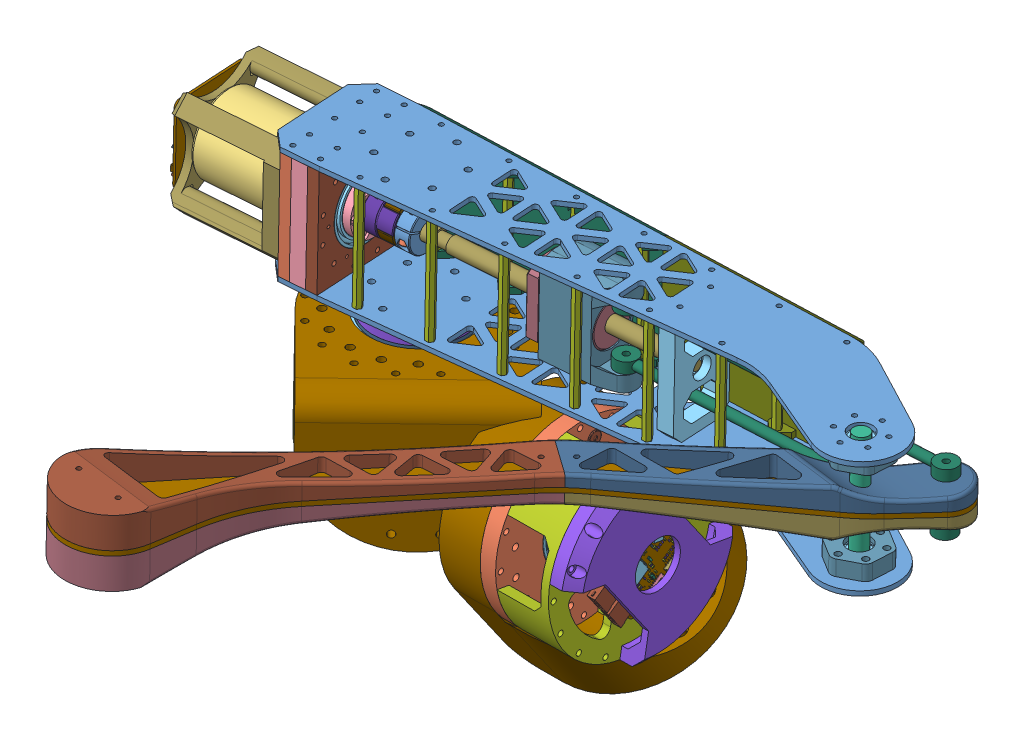
SolidWorks assembly Leg, configuration Default. Lengths in mm. (continued)
Components (placement in the parent): (continued)
- Cycloidal _v3-1: Cycloidal _v3 [Default] at (201.9883 83.8715 287.662) x (0.007254 0.020702 0.999759) z (-0.999974 0 0.007256) size (173.36 87.57 173.15) (continued)
  - M3x20-1: M3x20 [Default] at (43.4726 96.3558 90.1203) x (-0.837193 -0.000334 -0.546908) z (-0.546908 -0.000218 0.837193) size (6 21.2 6)
  - M3x10-1: M3x10 [Default] at (36.5111 25.853 142.5044) x (0.424034 0.000169 -0.905646) z (0.905646 0.000361 0.424034) size (6 11.2 6)
  - m3x60-1: m3x60 [Default] at (17.1068 35.0453 134.2855) x (-0.837193 -0.000334 -0.546908) z (-0.546908 -0.000218 0.837193) size (5.3 63 5.3)
  - m6-1: m6 [Default] at (60.6129 98.6627 108.4832) x (-0.153131 -0.000061 0.988206) z (0.988206 0.000394 0.153131) size (6 16 6)
- Cycloidal _v3-2: Cycloidal _v3 [Default] at (290.9356 44.932 396.0406) x (-0.007136 -0.180415 -0.983565) z (-0.001309 0.983591 -0.18041) size (173.36 87.57 173.15)
  - motor-X83008S.stp-1: motor-X83008S.stp [Default] at (3.9105 88.7742 94.1058) x (0.928336 0.00037 -0.371741) z (0.000399 -1 0) size (114.7 114.7 37.62) (hidden)
    - base.stp-1: base.stp [Default] at (42.0794 12.0269 46.7342) size (91.6 91.6 15.61)
    - stator.stp-1: stator.stp [Default] at (42.0794 12.0269 33.1342) x (0.08493 -0.996387 0) z (0 0 1) size (83 83 8)
    - coil.stp-1: coil.stp [Default] at (39.5332 41.8984 37.1342) x (0.996387 0.08493 0) z (-0.08493 0.996387 0) size (4.4 10.2 10.5)
    - coil.stp-2: coil.stp [Default] at (34.3848 41.0025 37.1342) x (0.966502 0.256661 0) z (-0.256661 0.966502 0) size (4.4 10.2 10.5)
    - coil.stp-3: coil.stp [Default] at (29.4701 39.2261 37.1342) x (0.90725 0.420593 0) z (-0.420593 0.90725 0) size (4.4 10.2 10.5)
    - coil.stp-4: coil.stp [Default] at (24.9386 36.6233 37.1342) x (0.820431 0.571745 0) z (-0.571745 0.820431 0) size (4.4 10.2 10.5)
    - coil.stp-5: coil.stp [Default] at (20.9279 33.2732 37.1342) x (0.708685 0.705525 0) z (-0.705525 0.708685 0) size (4.4 10.2 10.5)
    - coil.stp-6: coil.stp [Default] at (17.5599 29.2775 37.1342) x (0.575405 0.817869 0) z (-0.817869 0.575405 0) size (4.4 10.2 10.5)
    - coil.stp-7: coil.stp [Default] at (14.9368 24.7576 37.1342) x (0.424642 0.905361 0) z (-0.905361 0.424642 0) size (4.4 10.2 10.5)
    - coil.stp-8: coil.stp [Default] at (13.1385 19.8509 37.1342) x (0.260976 0.965345 0) z (-0.965345 0.260976 0) size (4.4 10.2 10.5)
    - coil.stp-9: coil.stp [Default] at (12.2196 14.7066 37.1342) x (0.089381 0.995998 0) z (-0.995998 0.089381 0) size (4.4 10.2 10.5)
    - coil.stp-10: coil.stp [Default] at (12.2079 9.4807 37.1342) x (-0.08493 0.996387 0) z (-0.996387 -0.08493 0) size (4.4 10.2 10.5)
    - coil.stp-11: coil.stp [Default] at (13.1039 4.3323 37.1342) x (-0.256661 0.966502 0) z (-0.966502 -0.256661 0) size (4.4 10.2 10.5)
    - coil.stp-12: coil.stp [Default] at (14.8802 -0.5824 37.1342) x (-0.420593 0.90725 0) z (-0.90725 -0.420593 0) size (4.4 10.2 10.5)
    - coil.stp-13: coil.stp [Default] at (17.483 -5.1139 37.1342) x (-0.571745 0.820431 0) z (-0.820431 -0.571745 0) size (4.4 10.2 10.5)
    - coil.stp-14: coil.stp [Default] at (20.8332 -9.1246 37.1342) x (-0.705525 0.708685 0) z (-0.708685 -0.705525 0) size (4.4 10.2 10.5)
    - coil.stp-15: coil.stp [Default] at (24.8289 -12.4926 37.1342) x (-0.817869 0.575405 0) z (-0.575405 -0.817869 0) size (4.4 10.2 10.5)
    - coil.stp-16: coil.stp [Default] at (29.3487 -15.1157 37.1342) x (-0.905361 0.424642 0) z (-0.424642 -0.905361 0) size (4.4 10.2 10.5)
    - coil.stp-17: coil.stp [Default] at (34.2554 -16.914 37.1342) x (-0.965345 0.260976 0) z (-0.260976 -0.965345 0) size (4.4 10.2 10.5)
    - coil.stp-18: coil.stp [Default] at (39.3998 -17.8329 37.1342) x (-0.995998 0.089381 0) z (-0.089381 -0.995998 0) size (4.4 10.2 10.5)
    - coil.stp-19: coil.stp [Default] at (44.6256 -17.8446 37.1342) x (-0.996387 -0.08493 0) z (0.08493 -0.996387 0) size (4.4 10.2 10.5)
    - coil.stp-20: coil.stp [Default] at (49.7741 -16.9486 37.1342) x (-0.966502 -0.256661 0) z (0.256661 -0.966502 0) size (4.4 10.2 10.5)
    - coil.stp-21: coil.stp [Default] at (54.6887 -15.1723 37.1342) x (-0.90725 -0.420593 0) z (0.420593 -0.90725 0) size (4.4 10.2 10.5)
    - coil.stp-22: coil.stp [Default] at (59.2202 -12.5695 37.1342) x (-0.820431 -0.571745 0) z (0.571745 -0.820431 0) size (4.4 10.2 10.5)
    - coil.stp-23: coil.stp [Default] at (63.2309 -9.2193 37.1342) x (-0.708685 -0.705525 0) z (0.705525 -0.708685 0) size (4.4 10.2 10.5)
    - coil.stp-24: coil.stp [Default] at (66.599 -5.2236 37.1342) x (-0.575405 -0.817869 0) z (0.817869 -0.575405 0) size (4.4 10.2 10.5)
    - coil.stp-25: coil.stp [Default] at (69.222 -0.7038 37.1342) x (-0.424642 -0.905361 0) z (0.905361 -0.424642 0) size (4.4 10.2 10.5)
    - coil.stp-26: coil.stp [Default] at (71.0203 4.2029 37.1342) x (-0.260976 -0.965345 0) z (0.965345 -0.260976 0) size (4.4 10.2 10.5)
    - coil.stp-27: coil.stp [Default] at (71.9392 9.3473 37.1342) x (-0.089381 -0.995998 0) z (0.995998 -0.089381 0) size (4.4 10.2 10.5)
    - coil.stp-28: coil.stp [Default] at (71.9509 14.5731 37.1342) x (0.08493 -0.996387 0) z (0.996387 0.08493 0) size (4.4 10.2 10.5)
    - coil.stp-29: coil.stp [Default] at (71.055 19.7216 37.1342) x (0.256661 -0.966502 0) z (0.966502 0.256661 0) size (4.4 10.2 10.5)
    - coil.stp-30: coil.stp [Default] at (69.2786 24.6362 37.1342) x (0.420593 -0.90725 0) z (0.90725 0.420593 0) size (4.4 10.2 10.5)
    - coil.stp-31: coil.stp [Default] at (66.6758 29.1677 37.1342) x (0.571745 -0.820431 0) z (0.820431 0.571745 0) size (4.4 10.2 10.5)
    - coil.stp-32: coil.stp [Default] at (63.3257 33.1785 37.1342) x (0.705525 -0.708685 0) z (0.708685 0.705525 0) size (4.4 10.2 10.5)
    - coil.stp-33: coil.stp [Default] at (59.33 36.5465 37.1342) x (0.817869 -0.575405 0) z (0.575405 0.817869 0) size (4.4 10.2 10.5)
    - coil.stp-34: coil.stp [Default] at (54.8101 39.1695 37.1342) x (0.905361 -0.424642 0) z (0.424642 0.905361 0) size (4.4 10.2 10.5)
    - coil.stp-35: coil.stp [Default] at (49.9034 40.9678 37.1342) x (0.965345 -0.260976 0) z (0.260976 0.965345 0) size (4.4 10.2 10.5)
    - coil.stp-36: coil.stp [Default] at (44.759 41.8868 37.1342) x (0.995998 -0.089381 0) z (0.089381 0.995998 0) size (4.4 10.2 10.5)
    - rotor.stp-1: rotor.stp [Default] at (42.0794 12.0269 42.1342) x (-0.293442 0.955977 0) z (0 0 -1) size (91.8 91.8 12)
    - outrunner.stp-1: outrunner.stp [Default] at (42.0794 12.0269 30.1342) x (-0.254711 0.967017 0) z (-0.967017 -0.254711 0) size (91.8 17.01 91.8)
    - screw-mount.stp-1: screw-mount.stp [Default] at (38.1314 27.0157 27.1342) x (1 0 0) z (0 0 -1) size (7 7 6.5)
    - screw-mount.stp-2: screw-mount.stp [Default] at (27.0906 8.0789 27.1342) x (1 0 0) z (0 0 -1) size (7 7 6.5)
    - screw-mount.stp-3: screw-mount.stp [Default] at (57.0682 15.9749 27.1342) x (1 0 0) z (0 0 -1) size (7 7 6.5)
    - screw-mount.stp-4: screw-mount.stp [Default] at (46.0274 -2.9618 27.1342) x (1 0 0) z (0 0 -1) size (7 7 6.5)
    - 6702ZZ-bearing-15x21x4.stp-1: 6702ZZ-bearing-15x21x4.stp [Default] at (42.0794 12.0269 43.7342) x (1 0 0) z (0 -1 0) size (21 4 21)
    - 6702ZZ-bearing-15x21x4.stp-2: 6702ZZ-bearing-15x21x4.stp [Default] at (42.0794 12.0269 35.1342) x (1 0 0) z (0 1 0) size (21 4 21)
    - shaft.stp-1: shaft.stp [Default] at (42.0794 12.0269 20.1342) size (16 16 31.6)
    - fix-screw.stp-1: fix-screw.stp [Default] at (42.0794 12.0269 51.7342) x (1 0 0) z (0 0 -1) size (19.67 18.96 12.02)
  - Base_Plate-1: Base_Plate [Default] at (47.4533 68.6574 89.6282) x (-0.992404 -0.000396 0.123023) z (-0.123023 -0.000049 -0.992404) size (39.8 11 39.8)
  - Eccentric_Shaft-1: Eccentric_Shaft [Default] at (60.4961 73.3217 80.3225) x (0.123023 0.000049 0.992404) z (-0.992404 -0.000396 0.123023) size (20 17 17)
    - Eccentric_Shaft_bot-1: Eccentric_Shaft_bot [Default] at (7.6302 12.3409 14.0904) x (1 0 0) z (0 0 -1) size (17 6 17)
    - Eccentric_Shaft_bot-2: Eccentric_Shaft_bot [Default] at (7.6302 12.3409 14.0904) x (-1 0 0) z (0 0 -1) size (17 6 17)
    - Eccentric_Shaft_top-1: Eccentric_Shaft_top [Default] at (7.6302 18.3409 14.0904) x (-1 0 0) z (0 0 -1) size (17 5 17)
  - radial ball bearing_68_iso-39: radial ball bearing_68_iso [ISO 15 RBB - 1860 - 32,SI,NC,32_68] at (47.4409 99.6574 89.6282) x (0.000399 -1 0) z (-0.546908 -0.000218 0.837193) size (10 78 78)
  - radial ball bearing_68_iso-40: radial ball bearing_68_iso [ISO 15 RBB - 1840 - 32,SI,NC,32_68] at (47.4516 72.9574 89.6282) x (-0.000399 1 0) z (0.001003 0 0.999999) size (7 52 52)
  - Base_plate_2-1: Base_plate_2 [Default] at (47.4529 69.6574 89.6282) x (0.712755 0.000284 -0.701413) z (0.701413 0.00028 0.712755) size (115 10 115)
  - m13_bearing-31: m13_bearing [Default] at (-10.4263 95.4017 67.196) x (0.227678 0.000091 0.973736) z (0.973736 0.000388 -0.227678) size (13 16 13)
    - m6-1: m6 [Default] at (8.4921 2.5508 14.8914) size (6 16 6)
    - radial ball bearing_68_iso-1: radial ball bearing_68_iso [ISO 15 RBB - 286 - 10,SI,NC,10_68] at (8.4921 16.0508 14.8914) x (0 1 0) z (0 0 1) size (5 13 13)
    - radial ball bearing_68_iso-2: radial ball bearing_68_iso [ISO 15 RBB - 286 - 10,SI,NC,10_68] at (8.4921 11.0508 14.8914) x (0 1 0) z (0 0 1) size (5 13 13)
  - m13_bearing-32: m13_bearing [Default] at (-13.9908 98.1837 84.3887) x (0.227678 0.000091 0.973736) z (0.973736 0.000388 -0.227678) size (13 16 13)
    - m6-1: m6 [Default] at (8.4921 2.5508 14.8914) size (6 16 6)
    - radial ball bearing_68_iso-1: radial ball bearing_68_iso [ISO 15 RBB - 286 - 10,SI,NC,10_68] at (8.4921 16.0508 14.8914) x (0 1 0) z (0 0 1) size (5 13 13)
    - radial ball bearing_68_iso-2: radial ball bearing_68_iso [ISO 15 RBB - 286 - 10,SI,NC,10_68] at (8.4921 11.0508 14.8914) x (0 1 0) z (0 0 1) size (5 13 13)
  - m13_bearing-34: m13_bearing [Default] at (13.4541 98.1947 126.1847) x (0.227678 0.000091 0.973736) z (0.973736 0.000388 -0.227678) size (13 16 13)
    - m6-1: m6 [Default] at (8.4921 2.5508 14.8914) size (6 16 6)
    - radial ball bearing_68_iso-1: radial ball bearing_68_iso [ISO 15 RBB - 286 - 10,SI,NC,10_68] at (8.4921 16.0508 14.8914) x (0 1 0) z (0 0 1) size (5 13 13)
    - radial ball bearing_68_iso-2: radial ball bearing_68_iso [ISO 15 RBB - 286 - 10,SI,NC,10_68] at (8.4921 11.0508 14.8914) x (0 1 0) z (0 0 1) size (5 13 13)
  - m13_bearing-35: m13_bearing [Default] at (-1.0662 98.1889 116.3132) x (0.227678 0.000091 0.973736) z (0.973736 0.000388 -0.227678) size (13 16 13)
    - m6-1: m6 [Default] at (8.4921 2.5508 14.8914) size (6 16 6)
    - radial ball bearing_68_iso-1: radial ball bearing_68_iso [ISO 15 RBB - 286 - 10,SI,NC,10_68] at (8.4921 16.0508 14.8914) x (0 1 0) z (0 0 1) size (5 13 13)
    - radial ball bearing_68_iso-2: radial ball bearing_68_iso [ISO 15 RBB - 286 - 10,SI,NC,10_68] at (8.4921 11.0508 14.8914) x (0 1 0) z (0 0 1) size (5 13 13)
  - m13_bearing-36: m13_bearing [Default] at (-10.7036 98.185 101.6364) x (0.227678 0.000091 0.973736) z (0.973736 0.000388 -0.227678) size (13 16 13)
    - m6-1: m6 [Default] at (8.4921 2.5508 14.8914) size (6 16 6)
    - radial ball bearing_68_iso-1: radial ball bearing_68_iso [ISO 15 RBB - 286 - 10,SI,NC,10_68] at (8.4921 16.0508 14.8914) x (0 1 0) z (0 0 1) size (5 13 13)
    - radial ball bearing_68_iso-2: radial ball bearing_68_iso [ISO 15 RBB - 286 - 10,SI,NC,10_68] at (8.4921 11.0508 14.8914) x (0 1 0) z (0 0 1) size (5 13 13)
  - m13_bearing-1: m13_bearing [Default] at (-0.4494 98.1891 62.778) x (0.736525 0.000294 0.676411) z (0.676411 0.00027 -0.736525) size (13 16 13)
    - m6-1: m6 [Default] at (8.4921 2.5508 14.8914) size (6 16 6)
    - radial ball bearing_68_iso-1: radial ball bearing_68_iso [ISO 15 RBB - 286 - 10,SI,NC,10_68] at (8.4921 16.0508 14.8914) x (0 1 0) z (0 0 1) size (5 13 13)
    - radial ball bearing_68_iso-2: radial ball bearing_68_iso [ISO 15 RBB - 286 - 10,SI,NC,10_68] at (8.4921 11.0508 14.8914) x (0 1 0) z (0 0 1) size (5 13 13)
  - m13_bearing-2: m13_bearing [Default] at (48.5236 98.2087 124.7001) x (0.120271 0.000048 0.992741) z (0.992741 0.000396 -0.120271) size (13 16 13)
    - m6-1: m6 [Default] at (8.4921 2.5508 14.8914) size (6 16 6)
    - radial ball bearing_68_iso-1: radial ball bearing_68_iso [ISO 15 RBB - 286 - 10,SI,NC,10_68] at (8.4921 16.0508 14.8914) x (0 1 0) z (0 0 1) size (5 13 13)
    - radial ball bearing_68_iso-2: radial ball bearing_68_iso [ISO 15 RBB - 286 - 10,SI,NC,10_68] at (8.4921 11.0508 14.8914) x (0 1 0) z (0 0 1) size (5 13 13)
  - m13_bearing-3: m13_bearing [Default] at (32.5019 98.2023 52.3604) x (0.833889 0.000333 0.551933) z (0.551932 0.00022 -0.833889) size (13 16 13)
    - m6-1: m6 [Default] at (8.4921 2.5508 14.8914) size (6 16 6)
    - radial ball bearing_68_iso-1: radial ball bearing_68_iso [ISO 15 RBB - 286 - 10,SI,NC,10_68] at (8.4921 16.0508 14.8914) x (0 1 0) z (0 0 1) size (5 13 13)
    - radial ball bearing_68_iso-2: radial ball bearing_68_iso [ISO 15 RBB - 286 - 10,SI,NC,10_68] at (8.4921 11.0508 14.8914) x (0 1 0) z (0 0 1) size (5 13 13)
  - m13_bearing-4: m13_bearing [Default] at (77.3632 98.2202 81.8307) x (0.022268 0.000009 0.999752) z (0.999752 0.000399 -0.022268) size (13 16 13)
    - m6-1: m6 [Default] at (8.4921 2.5508 14.8914) size (6 16 6)
    - radial ball bearing_68_iso-1: radial ball bearing_68_iso [ISO 15 RBB - 286 - 10,SI,NC,10_68] at (8.4921 16.0508 14.8914) x (0 1 0) z (0 0 1) size (5 13 13)
    - radial ball bearing_68_iso-2: radial ball bearing_68_iso [ISO 15 RBB - 286 - 10,SI,NC,10_68] at (8.4921 11.0508 14.8914) x (0 1 0) z (0 0 1) size (5 13 13)
  - m13_bearing-5: m13_bearing [Default] at (73.5091 98.2186 99.5852) x (0.059133 0.000024 0.99825) z (0.99825 0.000398 -0.059133) size (13 16 13)
    - m6-1: m6 [Default] at (8.4921 2.5508 14.8914) size (6 16 6)
    - radial ball bearing_68_iso-1: radial ball bearing_68_iso [ISO 15 RBB - 286 - 10,SI,NC,10_68] at (8.4921 16.0508 14.8914) x (0 1 0) z (0 0 1) size (5 13 13)
    - radial ball bearing_68_iso-2: radial ball bearing_68_iso [ISO 15 RBB - 286 - 10,SI,NC,10_68] at (8.4921 11.0508 14.8914) x (0 1 0) z (0 0 1) size (5 13 13)
  - m13_bearing-6: m13_bearing [Default] at (13.4333 98.1947 47.0643) x (0.451561 0.00018 0.89224) z (0.89224 0.000356 -0.451561) size (13 16 13)
    - m6-1: m6 [Default] at (8.4921 2.5508 14.8914) size (6 16 6)
    - radial ball bearing_68_iso-1: radial ball bearing_68_iso [ISO 15 RBB - 286 - 10,SI,NC,10_68] at (8.4921 16.0508 14.8914) x (0 1 0) z (0 0 1) size (5 13 13)
    - radial ball bearing_68_iso-2: radial ball bearing_68_iso [ISO 15 RBB - 286 - 10,SI,NC,10_68] at (8.4921 11.0508 14.8914) x (0 1 0) z (0 0 1) size (5 13 13)
  - m13_bearing-7: m13_bearing [Default] at (57.1526 98.2121 32.9496) x (-0.545813 -0.000218 0.837907) z (0.837907 0.000334 0.545813) size (13 16 13)
    - m6-1: m6 [Default] at (8.4921 2.5508 14.8914) size (6 16 6)
    - radial ball bearing_68_iso-1: radial ball bearing_68_iso [ISO 15 RBB - 286 - 10,SI,NC,10_68] at (8.4921 16.0508 14.8914) x (0 1 0) z (0 0 1) size (5 13 13)
    - radial ball bearing_68_iso-2: radial ball bearing_68_iso [ISO 15 RBB - 286 - 10,SI,NC,10_68] at (8.4921 11.0508 14.8914) x (0 1 0) z (0 0 1) size (5 13 13)
  - m13_bearing-8: m13_bearing [Default] at (73.1034 98.2185 66.7178) x (0.158553 0.000063 0.98735) z (0.98735 0.000394 -0.158553) size (13 16 13)
    - m6-1: m6 [Default] at (8.4921 2.5508 14.8914) size (6 16 6)
    - radial ball bearing_68_iso-1: radial ball bearing_68_iso [ISO 15 RBB - 286 - 10,SI,NC,10_68] at (8.4921 16.0508 14.8914) x (0 1 0) z (0 0 1) size (5 13 13)
    - radial ball bearing_68_iso-2: radial ball bearing_68_iso [ISO 15 RBB - 286 - 10,SI,NC,10_68] at (8.4921 11.0508 14.8914) x (0 1 0) z (0 0 1) size (5 13 13)
  - m13_bearing-9: m13_bearing [Default] at (74.5316 98.219 41.6624) x (-0.687134 -0.000274 0.72653) z (0.72653 0.00029 0.687134) size (13 16 13)
    - m6-1: m6 [Default] at (8.4921 2.5508 14.8914) size (6 16 6)
    - radial ball bearing_68_iso-1: radial ball bearing_68_iso [ISO 15 RBB - 286 - 10,SI,NC,10_68] at (8.4921 16.0508 14.8914) x (0 1 0) z (0 0 1) size (5 13 13)
    - radial ball bearing_68_iso-2: radial ball bearing_68_iso [ISO 15 RBB - 286 - 10,SI,NC,10_68] at (8.4921 11.0508 14.8914) x (0 1 0) z (0 0 1) size (5 13 13)
  - m13_bearing-11: m13_bearing [Default] at (30.0113 98.2013 136.2104) x (0.57351 0.000229 0.819198) z (0.819198 0.000327 -0.57351) size (13 16 13)
    - m6-1: m6 [Default] at (8.4921 2.5508 14.8914) size (6 16 6)
    - radial ball bearing_68_iso-1: radial ball bearing_68_iso [ISO 15 RBB - 286 - 10,SI,NC,10_68] at (8.4921 16.0508 14.8914) x (0 1 0) z (0 0 1) size (5 13 13)
    - radial ball bearing_68_iso-2: radial ball bearing_68_iso [ISO 15 RBB - 286 - 10,SI,NC,10_68] at (8.4921 11.0508 14.8914) x (0 1 0) z (0 0 1) size (5 13 13)
  - m13_bearing-12: m13_bearing [Default] at (62.5932 98.2143 116.7506) x (0.22335 0.000089 0.974738) z (0.974738 0.000389 -0.22335) size (13 16 13)
    - m6-1: m6 [Default] at (8.4921 2.5508 14.8914) size (6 16 6)
    - radial ball bearing_68_iso-1: radial ball bearing_68_iso [ISO 15 RBB - 286 - 10,SI,NC,10_68] at (8.4921 16.0508 14.8914) x (0 1 0) z (0 0 1) size (5 13 13)
    - radial ball bearing_68_iso-2: radial ball bearing_68_iso [ISO 15 RBB - 286 - 10,SI,NC,10_68] at (8.4921 11.0508 14.8914) x (0 1 0) z (0 0 1) size (5 13 13)
  - M3x4x4.2_brass_insert-22: M3x4x4.2_brass_insert [Default] at (43.4837 68.6558 90.1203) x (0.984609 0.000393 -0.174769) z (0.174769 0.00007 0.984609) size (4 4 4)
  - M3x4x4.2_brass_insert-23: M3x4x4.2_brass_insert [Default] at (51.4229 68.659 89.1361) x (0.984609 0.000393 -0.174769) z (0.174769 0.00007 0.984609) size (4 4 4)
  - radial ball bearing_68_iso-44: radial ball bearing_68_iso [ISO 15 RBB - 1715 - 26,SI,NC,26_68] at (47.2636 81.6573 88.1396) x (0.000399 -1 0) z (0.171535 0.000068 0.985178) size (4 21 21)
  - radial ball bearing_68_iso-45: radial ball bearing_68_iso [ISO 15 RBB - 1715 - 26,SI,NC,26_68] at (47.4429 94.6574 89.6282) x (0.000399 -1 0) z (0.819169 0.000327 0.573552) size (4 21 21)
  - radial ball bearing_68_iso-46: radial ball bearing_68_iso [ISO 15 RBB - 1715 - 26,SI,NC,26_68] at (47.6295 89.6575 91.1168) x (-0.000399 1 0) z (0 0 1) size (4 21 21)
  - foc-motor-controller.step-1: foc-motor-controller.step [Default] at (47.4677 32.6574 89.6282) x (0.701413 0.00028 0.712755) z (0.000399 -1 0) size (57.23 50 8.13)
    - RTA0040B.step-1: RTA0040B.step [Default] at (12.5014 -1.6986 1.595) x (-0.707107 -0.707107 0) z (0 0 1) size (6 6 1)
      - FRAME.step-1: FRAME.step [Default] x (1 0 0) z (0 -1 0) size (6 0.2 6)
        - SOLID.step-1: SOLID.step [Default] at origin size (0.4 0.2 0.22)
        - SOLID-0.step-1: SOLID-0.step [Default] at origin size (0.4 0.2 0.22)
        - SOLID-1.step-1: SOLID-1.step [Default] at origin size (0.4 0.2 0.22)
        - SOLID-2.step-1: SOLID-2.step [Default] at origin size (0.4 0.2 0.22)
        - SOLID-3.step-1: SOLID-3.step [Default] at origin size (0.4 0.2 0.22)
        - SOLID-4.step-1: SOLID-4.step [Default] at origin size (0.4 0.2 0.22)
        - SOLID-5.step-1: SOLID-5.step [Default] at origin size (0.4 0.2 0.22)
        - SOLID-6.step-1: SOLID-6.step [Default] at origin size (0.4 0.2 0.22)
        - SOLID-7.step-1: SOLID-7.step [Default] at origin size (0.4 0.2 0.22)
        - SOLID-8.step-1: SOLID-8.step [Default] at origin size (0.4 0.2 0.22)
        - SOLID-9.step-1: SOLID-9.step [Default] at origin size (0.22 0.2 0.4)
        - SOLID-10.step-1: SOLID-10.step [Default] at origin size (0.22 0.2 0.4)
        - SOLID-11.step-1: SOLID-11.step [Default] at origin size (0.22 0.2 0.4)
        - SOLID-12.step-1: SOLID-12.step [Default] at origin size (0.22 0.2 0.4)
        - SOLID-13.step-1: SOLID-13.step [Default] at origin size (0.22 0.2 0.4)
        - SOLID-14.step-1: SOLID-14.step [Default] at origin size (0.22 0.2 0.4)
        - SOLID-15.step-1: SOLID-15.step [Default] at origin size (0.22 0.2 0.4)
        - SOLID-16.step-1: SOLID-16.step [Default] at origin size (0.22 0.2 0.4)
        - SOLID-17.step-1: SOLID-17.step [Default] at origin size (4.15 0.2 4.15)
        - SOLID-18.step-1: SOLID-18.step [Default] at origin size (0.28 0.1 0.28)
        - SOLID-19.step-1: SOLID-19.step [Default] at origin size (0.28 0.1 0.28)
        - SOLID-20.step-1: SOLID-20.step [Default] at origin size (0.28 0.1 0.28)
        - SOLID-21.step-1: SOLID-21.step [Default] at origin size (0.28 0.1 0.28)
        - SOLID-22.step-1: SOLID-22.step [Default] at origin size (0.4 0.2 0.22)
        - SOLID-23.step-1: SOLID-23.step [Default] at origin size (0.4 0.2 0.22)
        - SOLID-24.step-1: SOLID-24.step [Default] at origin size (0.4 0.2 0.22)
        - SOLID-25.step-1: SOLID-25.step [Default] at origin size (0.4 0.2 0.22)
        - SOLID-26.step-1: SOLID-26.step [Default] at origin size (0.4 0.2 0.22)
        - SOLID-27.step-1: SOLID-27.step [Default] at origin size (0.4 0.2 0.22)
        - SOLID-28.step-1: SOLID-28.step [Default] at origin size (0.4 0.2 0.22)
        - SOLID-29.step-1: SOLID-29.step [Default] at origin size (0.4 0.2 0.22)
        - SOLID-30.step-1: SOLID-30.step [Default] at origin size (0.4 0.2 0.22)
        - SOLID-31.step-1: SOLID-31.step [Default] at origin size (0.4 0.2 0.22)
        - SOLID-32.step-1: SOLID-32.step [Default] at origin size (0.22 0.2 0.4)
        - SOLID-33.step-1: SOLID-33.step [Default] at origin size (0.22 0.2 0.4)
        - SOLID-34.step-1: SOLID-34.step [Default] at origin size (0.22 0.2 0.4)
        - SOLID-35.step-1: SOLID-35.step [Default] at origin size (0.22 0.2 0.4)
        - SOLID-36.step-1: SOLID-36.step [Default] at origin size (0.22 0.2 0.4)
        - SOLID-37.step-1: SOLID-37.step [Default] at origin size (0.22 0.2 0.4)
        - SOLID-38.step-1: SOLID-38.step [Default] at origin size (0.22 0.2 0.4)
        - SOLID-39.step-1: SOLID-39.step [Default] at origin size (0.22 0.2 0.4)
        - SOLID-40.step-1: SOLID-40.step [Default] at origin size (0.22 0.2 0.4)
        - SOLID-41.step-1: SOLID-41.step [Default] at origin size (0.22 0.2 0.4)
        - SOLID-42.step-1: SOLID-42.step [Default] at origin size (0.22 0.2 0.4)
        - SOLID-43.step-1: SOLID-43.step [Default] at origin size (0.22 0.2 0.4)
      - BODY.step-1: BODY.step [Default] at (0 0 0.025) x (1 0 0) z (0 -1 0) size (6 0.97 6)
    - Resonator_SMD_Murata_CSTxExxV-3Pin_3.0x1.1mm.step-1: Resonator_SMD_Murata_CSTxExxV-3Pin_3.0x1.1mm.step [Default] at (1.8 -7 1.595) x (0 1 0) z (0 0 1) size (3.2 1.35 0.9)
    - C_0603_1608Metric.step-1: C_0603_1608Metric.step [Default] at (6.2 -16.8 1.595) x (0 -1 0) z (0 0 1) size (1.6 0.8 0.8)
    - R_0603_1608Metric.step-1: R_0603_1608Metric.step [Default] at (11.8 -7.375 1.595) x (0 1 0) z (0 0 1) size (1.6 0.8 0.45)
    - R_0603_1608Metric.step-2: R_0603_1608Metric.step [Default] at (13.8 -16.8 1.595) x (0 1 0) z (0 0 1) size (1.6 0.8 0.45)
    - R_0603_1608Metric.step-3: R_0603_1608Metric.step [Default] at (18.1 -5.36 1.595) size (1.6 0.8 0.45)
    - C_0603_1608Metric.step-2: C_0603_1608Metric.step [Default] at (2.6 -0.5 1.595) x (0 -1 0) z (0 0 1) size (1.6 0.8 0.8)
    - R_0603_1608Metric.step-4: R_0603_1608Metric.step [Default] at (14.6 -11.3 1.595) x (0 1 0) z (0 0 1) size (1.6 0.8 0.45)
    - L_APV_ANR4020.step-1: L_APV_ANR4020.step [Default] at (22.3 -13.7 1.595) x (0 -1 0) z (0 0 1) size (4.02 4 2)
    - C_0603_1608Metric.step-3: C_0603_1608Metric.step [Default] at (0.3 -12.6 1.595) x (-1 0 0) z (0 0 1) size (1.6 0.8 0.8)
    - C_1206_3216Metric.step-1: C_1206_3216Metric.step [Default] at (15.7 11 1.595) x (0 1 0) z (0 0 1) size (3.2 1.6 1.6)
    - C_0603_1608Metric.step-4: C_0603_1608Metric.step [Default] at (0.3 -9.6 1.595) size (1.6 0.8 0.8)
    - R_0603_1608Metric.step-5: R_0603_1608Metric.step [Default] at (12.3 -16.8 1.595) x (0 1 0) z (0 0 1) size (1.6 0.8 0.45)
    - C_0603_1608Metric.step-5: C_0603_1608Metric.step [Default] at (-0.3 -16.6 1.595) x (0 1 0) z (0 0 1) size (1.6 0.8 0.8)
    - R_0603_1608Metric.step-6: R_0603_1608Metric.step [Default] at (10.9 4.1 1.595) size (1.6 0.8 0.45)
    - C_1206_3216Metric.step-2: C_1206_3216Metric.step [Default] at (6.3 11 1.595) x (0 1 0) z (0 0 1) size (3.2 1.6 1.6)
    - XT30PW_2_2_-M.G.B.step-1: XT30PW_2_2_-M.G.B.step [Default] at (-20.5 9.5 1.595) x (0 -1 0) z (-1 0 0) size (15.5 7.1 12.53)
    - R_0603_1608Metric.step-7: R_0603_1608Metric.step [Default] at (0.3 -11.1 1.595) size (1.6 0.8 0.45)
    - C_0603_1608Metric.step-6: C_0603_1608Metric.step [Default] at (19 -0.4 1.595) x (-0.707107 -0.707107 0) z (0 0 1) size (1.6 0.8 0.8)
    - C_1206_3216Metric.step-3: C_1206_3216Metric.step [Default] at (13.3 11 1.595) x (0 1 0) z (0 0 1) size (3.2 1.6 1.6)
    - R_0603_1608Metric.step-8: R_0603_1608Metric.step [Default] at (10.2 -7.375 1.595) x (0 -1 0) z (0 0 1) size (1.6 0.8 0.45)
    - JST_GH_SM08B-GHS-TB_1x08-1MP_P1.25mm_Horizontal.step-1: JST_GH_SM08B-GHS-TB_1x08-1MP_P1.25mm_Horizontal.step [Default] at (10 -22 1.595) size (13.25 4.95 4.25)
    - C_1206_3216Metric.step-4: C_1206_3216Metric.step [Default] at (-12.3 11 1.595) x (0 1 0) z (0 0 1) size (3.2 1.6 1.6)
    - JST_GH_SM06B-GHS-TB_1x06-1MP_P1.25mm_Horizontal.step-1: JST_GH_SM06B-GHS-TB_1x06-1MP_P1.25mm_Horizontal.step [Default] at (-4.3 -22 1.595) size (10.75 4.95 4.25)
    - C_0603_1608Metric.step-7: C_0603_1608Metric.step [Default] at (7.3 -4.5 1.595) x (-1 0 0) z (0 0 1) size (1.6 0.8 0.8)
    - R_0603_1608Metric.step-9: R_0603_1608Metric.step [Default] at (18.1 -3.86 1.595) x (-1 0 0) z (0 0 1) size (1.6 0.8 0.45)
    - C_1206_3216Metric.step-5: C_1206_3216Metric.step [Default] at (22.6794 -1.2206 1.595) x (0.707107 -0.707107 0) z (0 0 1) size (3.2 1.6 1.6)
    - R_Array_Convex_4x0402.step-1: R_Array_Convex_4x0402.step [Default] at (6.8 -2.5 1.595) size (1 2 0.35)
    - R_0603_1608Metric.step-10: R_0603_1608Metric.step [Default] at (7.7 -16.8 1.595) x (0 -1 0) z (0 0 1) size (1.6 0.8 0.45)
    - C_1206_3216Metric.step-6: C_1206_3216Metric.step [Default] at (8.7 11 1.595) x (0 1 0) z (0 0 1) size (3.2 1.6 1.6)
    - C_0603_1608Metric.step-8: C_0603_1608Metric.step [Default] at (16.1 -11.3 1.595) x (0 1 0) z (0 0 1) size (1.6 0.8 0.8)
    - SOT-23-5.step-1: SOT-23-5.step [Default] at (-3.1 -16.6 1.595) x (-1 0 0) z (0 0 1) size (2.8 2.9 1.55)
    - C_0603_1608Metric.step-9: C_0603_1608Metric.step [Default] at (17.8 -13.6 1.595) size (1.6 0.8 0.8)
    - R_0603_1608Metric.step-11: R_0603_1608Metric.step [Default] at (-11.5 -20.3875 1.595) x (0 -1 0) z (0 0 1) size (1.6 0.8 0.45)
    - C_0603_1608Metric.step-10: C_0603_1608Metric.step [Default] at (-12.4 2.3 1.595) x (0 1 0) z (0 0 1) size (1.6 0.8 0.8)
    - C_1206_3216Metric.step-7: C_1206_3216Metric.step [Default] at (18 11 1.595) x (0 1 0) z (0 0 1) size (3.2 1.6 1.6)
    - R_0603_1608Metric.step-12: R_0603_1608Metric.step [Default] at (-10.8105 -14.9971 1.595) x (-1 0 0) z (0 0 1) size (1.6 0.8 0.45)
    - C_0603_1608Metric.step-11: C_0603_1608Metric.step [Default] at (-13.8 -9.4 1.595) x (-1 0 0) z (0 0 1) size (1.6 0.8 0.8)
    - R_0603_1608Metric.step-13: R_0603_1608Metric.step [Default] at (-23.15 -14.5 1.595) x (-1 0 0) z (0 0 1) size (1.6 0.8 0.45)
    - C_0603_1608Metric.step-12: C_0603_1608Metric.step [Default] at (1.1 -0.2 1.595) x (0 1 0) z (0 0 1) size (1.6 0.8 0.8)
    - D_0805_2012Metric.step-1: D_0805_2012Metric.step [Default] at (22.9 -9.6 1.595) x (0 1 0) z (0 0 1) size (2 1.27 0.8)
    - C_0603_1608Metric.step-13: C_0603_1608Metric.step [Default] at (-7.8 3.775 1.595) x (0 -1 0) z (0 0 1) size (1.6 0.8 0.8)
    - R_0603_1608Metric.step-14: R_0603_1608Metric.step [Default] at (-6.4 -12.825 1.595) x (0 1 0) z (0 0 1) size (1.6 0.8 0.45)
    - L_0603_1608Metric.step-1: L_0603_1608Metric.step [Default] at (-10.1 3 1.595) size (1.6 0.8 0.8)
    - C_0603_1608Metric.step-14: C_0603_1608Metric.step [Default] at (17.9 0.7 1.595) x (-0.707107 -0.707107 0) z (0 0 1) size (1.6 0.8 0.8)
    - HVSSOP-10.step-1: HVSSOP-10.step [Default] at (18.6 -9.6 1.595) x (0 -1 0) z (-1 0 0) size (4.9 1.1 3)
    - C_0603_1608Metric.step-15: C_0603_1608Metric.step [Default] at (7.9 4.1 1.595) x (-1 0 0) z (0 0 1) size (1.6 0.8 0.8)
    - C_0603_1608Metric.step-16: C_0603_1608Metric.step [Default] at (21.1 -9.6 1.595) x (0 -1 0) z (0 0 1) size (1.6 0.8 0.8)
    - R_0603_1608Metric.step-15: R_0603_1608Metric.step [Default] at (-10.8105 -11.9971 1.595) x (-1 0 0) z (0 0 1) size (1.6 0.8 0.45)
    - R_0603_1608Metric.step-16: R_0603_1608Metric.step [Default] at (-18.2 -17.4 1.595) size (1.6 0.8 0.45)
    - C_1206_3216Metric.step-8: C_1206_3216Metric.step [Default] at (-3 11 1.595) x (0 1 0) z (0 0 1) size (3.2 1.6 1.6)
    - R_0603_1608Metric.step-17: R_0603_1608Metric.step [Default] at (-16.9 -20.4 1.595) x (0 -1 0) z (0 0 1) size (1.6 0.8 0.45)
    - R_0603_1608Metric.step-18: R_0603_1608Metric.step [Default] at (-13.3 -20.3875 1.595) x (0 -1 0) z (0 0 1) size (1.6 0.8 0.45)
    - R_0603_1608Metric.step-19: R_0603_1608Metric.step [Default] at (-15.1 -20.3875 1.595) x (0 -1 0) z (0 0 1) size (1.6 0.8 0.45)
    - C_0603_1608Metric.step-17: C_0603_1608Metric.step [Default] at (15.5 -14.4 1.595) x (0 -1 0) z (0 0 1) size (1.6 0.8 0.8)
    - LED_0603_1608Metric.step-1: LED_0603_1608Metric.step [Default] at (-11.5 -23.3875 1.595) x (0 1 0) z (0 0 1) size (1.6 0.8 1.1)
    - C_0805_2012Metric.step-1: C_0805_2012Metric.step [Default] at (19.95 -17 1.595) size (2 1.25 1.25)
    - D_SMB.step-1: D_SMB.step [Default] at (-16.5 11.208 1.595) x (0 -1 0) z (0 0 1) size (5.3 3.55 2.15)
    - C_1206_3216Metric.step-9: C_1206_3216Metric.step [Default] at (-5.3 11 1.595) x (0 1 0) z (0 0 1) size (3.2 1.6 1.6)
    - XT30PW_2_2_-M.G.B.step-2: XT30PW_2_2_-M.G.B.step [Default] at (-20.5 -6.5 1.595) x (0 -1 0) z (-1 0 0) size (15.5 7.1 12.53)
    - C_1206_3216Metric.step-10: C_1206_3216Metric.step [Default] at (1.7 11 1.595) x (0 1 0) z (0 0 1) size (3.2 1.6 1.6)
    - C_1206_3216Metric.step-11: C_1206_3216Metric.step [Default] at (11 11 1.595) x (0 1 0) z (0 0 1) size (3.2 1.6 1.6)
    - C_0603_1608Metric.step-18: C_0603_1608Metric.step [Default] at (-6.3 3.775 1.595) x (0 -1 0) z (0 0 1) size (1.6 0.8 0.8)
    - C_0603_1608Metric.step-19: C_0603_1608Metric.step [Default] at (16.8686 1.7314 1.595) x (0.707107 0.707107 0) z (0 0 1) size (1.6 0.8 0.8)
    - C_0603_1608Metric.step-20: C_0603_1608Metric.step [Default] at (-15.0105 -11.1 1.595) size (1.6 0.8 0.8)
    - C_1206_3216Metric.step-12: C_1206_3216Metric.step [Default] at (-7.7 11 1.595) x (0 1 0) z (0 0 1) size (3.2 1.6 1.6)
    - C_0603_1608Metric.step-21: C_0603_1608Metric.step [Default] at (-18.2 -15.8 1.595) size (1.6 0.8 0.8)
    - C_0603_1608Metric.step-22: C_0603_1608Metric.step [Default] at (-2.1 -11.3 1.595) x (0 -1 0) z (0 0 1) size (1.6 0.8 0.8)
    - C_0603_1608Metric.step-23: C_0603_1608Metric.step [Default] at (-10.8105 -13.4971 1.595) size (1.6 0.8 0.8)
    - C_1206_3216Metric.step-13: C_1206_3216Metric.step [Default] at (4 11 1.595) x (0 1 0) z (0 0 1) size (3.2 1.6 1.6)
    - R_0603_1608Metric.step-20: R_0603_1608Metric.step [Default] at (16 -17.8 1.595) x (0 1 0) z (0 0 1) size (1.6 0.8 0.45)
    - Texas_S-PVSON-N8.step-1: Texas_S-PVSON-N8.step [Default] at (-14.4105 -13.7 1.595) x (-1 0 0) z (0 0 1) size (3 2.98 0.92)
    - C_1206_3216Metric.step-14: C_1206_3216Metric.step [Default] at (21 -2.9 1.595) x (0.707107 -0.707107 0) z (0 0 1) size (3.2 1.6 1.6)
    - C_0603_1608Metric.step-24: C_0603_1608Metric.step [Default] at (-5.9 -16.6 1.595) x (0 1 0) z (0 0 1) size (1.6 0.8 0.8)
    - C_0603_1608Metric.step-25: C_0603_1608Metric.step [Default] at (-3.1 -14.1 1.595) size (1.6 0.8 0.8)
    - R_0603_1608Metric.step-21: R_0603_1608Metric.step [Default] at (7.2 -7.375 1.595) x (0 -1 0) z (0 0 1) size (1.6 0.8 0.45)
    - C_1206_3216Metric.step-15: C_1206_3216Metric.step [Default] at (-0.7 11 1.595) x (0 1 0) z (0 0 1) size (3.2 1.6 1.6)
    - LQFP-64_10x10mm_P0.5mm.step-1: LQFP-64_10x10mm_P0.5mm.step [Default] at (-7 -4.5 1.595) x (-1 0 0) z (0 0 1) size (12 12 1.5)
    - C_0805_2012Metric.step-2: C_0805_2012Metric.step [Default] at (23.35 -17 1.595) x (-1 0 0) z (0 0 1) size (2 1.25 1.25)
    - C_0603_1608Metric.step-26: C_0603_1608Metric.step [Default] at (10.8 -16.8 1.595) x (0 -1 0) z (0 0 1) size (1.6 0.8 0.8)
    - R_0603_1608Metric.step-22: R_0603_1608Metric.step [Default] at (17.5 -17.8 1.595) x (0 -1 0) z (0 0 1) size (1.6 0.8 0.45)
    - C_1206_3216Metric.step-16: C_1206_3216Metric.step [Default] at (20.3 11 1.595) x (0 1 0) z (0 0 1) size (3.2 1.6 1.6)
    - R_0603_1608Metric.step-23: R_0603_1608Metric.step [Default] at (9.2 -16.8 1.595) x (0 -1 0) z (0 0 1) size (1.6 0.8 0.45)
    - C_1206_3216Metric.step-17: C_1206_3216Metric.step [Default] at (-10 11 1.595) x (0 1 0) z (0 0 1) size (3.2 1.6 1.6)
    - R_0603_1608Metric.step-24: R_0603_1608Metric.step [Default] at (17.8 -15.2 1.595) size (1.6 0.8 0.45)
    - C_1206_3216Metric.step-18: C_1206_3216Metric.step [Default] at (19.9 2.6 1.595) x (-0.707107 0.707107 0) z (0 0 1) size (3.2 1.6 1.6)
    - C_0603_1608Metric.step-27: C_0603_1608Metric.step [Default] at (13.4 -7.375 1.595) x (0 -1 0) z (0 0 1) size (1.6 0.8 0.8)
    - R_0603_1608Metric.step-25: R_0603_1608Metric.step [Default] at (8.7 -7.375 1.595) x (0 -1 0) z (0 0 1) size (1.6 0.8 0.45)
    - PQFN-8-EP_6x5mm_P1.27mm_Generic.step-1: PQFN-8-EP_6x5mm_P1.27mm_Generic.step [Default] at (4.9 14.4 -0.085) x (0 1 0) z (0 0 -1) size (6.15 5.15 1.09)
    - C_0805_2012Metric.step-3: C_0805_2012Metric.step [Default] at (-3 8.9 -0.085) x (0 1 0) z (0 0 -1) size (2 1.25 1.25)
    - C_0603_1608Metric.step-28: C_0603_1608Metric.step [Default] at (1.5 -4.3 -0.085) x (0 1 0) z (0 0 -1) size (1.6 0.8 0.8)
    - R_2512_6332Metric.step-1: R_2512_6332Metric.step [Default] at (2.1 8.6 -0.085) x (-1 0 0) z (0 0 -1) size (6.3 3.2 0.6)
    - C_0805_2012Metric.step-4: C_0805_2012Metric.step [Default] at (18.8 8.9 -0.085) x (0 1 0) z (0 0 -1) size (2 1.25 1.25)
    - C_0805_2012Metric.step-5: C_0805_2012Metric.step [Default] at (-5.2 8.901 -0.085) x (0 1 0) z (0 0 -1) size (2 1.25 1.25)
    - PQFN-8-EP_6x5mm_P1.27mm_Generic.step-2: PQFN-8-EP_6x5mm_P1.27mm_Generic.step [Default] at (16.9 14.6 -0.085) x (0 -1 0) z (0 0 -1) size (6.15 5.15 1.09)
    - PQFN-8-EP_6x5mm_P1.27mm_Generic.step-3: PQFN-8-EP_6x5mm_P1.27mm_Generic.step [Default] at (-1.1 14.6 -0.085) x (0 -1 0) z (0 0 -1) size (6.15 5.15 1.09)
    - R_0603_1608Metric.step-26: R_0603_1608Metric.step [Default] at (8.2 8.8 -0.085) x (0 1 0) z (0 0 -1) size (1.6 0.8 0.45)
    - R_2512_6332Metric.step-2: R_2512_6332Metric.step [Default] at (-10.3 8.601 -0.085) x (1 0 0) z (0 0 -1) size (6.3 3.2 0.6)
    - TSSOP-16_4.4x5mm_P0.65mm.step-1: TSSOP-16_4.4x5mm_P0.65mm.step [Default] at (0 0 -0.085) x (-1 0 0) z (0 0 -1) size (6.4 5 1.1)
    - C_0603_1608Metric.step-29: C_0603_1608Metric.step [Default] at (0 -4.25 -0.085) x (0 1 0) z (0 0 -1) size (1.6 0.8 0.8)
    - PQFN-8-EP_6x5mm_P1.27mm_Generic.step-4: PQFN-8-EP_6x5mm_P1.27mm_Generic.step [Default] at (10.9 14.4 -0.085) x (0 1 0) z (0 0 -1) size (6.15 5.15 1.09)
    - R_2512_6332Metric.step-3: R_2512_6332Metric.step [Default] at (13.7 8.6 -0.085) x (1 0 0) z (0 0 -1) size (6.3 3.2 0.6)
    - PQFN-8-EP_6x5mm_P1.27mm_Generic.step-5: PQFN-8-EP_6x5mm_P1.27mm_Generic.step [Default] at (-13.1 14.401 -0.085) x (0 1 0) z (0 0 -1) size (6.15 5.15 1.09)
    - C_0603_1608Metric.step-30: C_0603_1608Metric.step [Default] at (-1.5 -4.3 -0.085) x (0 -1 0) z (0 0 -1) size (1.6 0.8 0.8)
    - PQFN-8-EP_6x5mm_P1.27mm_Generic.step-6: PQFN-8-EP_6x5mm_P1.27mm_Generic.step [Default] at (-7.1 14.601 -0.085) x (0 -1 0) z (0 0 -1) size (6.15 5.15 1.09)
    - foc-motor-controller_PCB.step-1: foc-motor-controller_PCB.step [Default] at origin size (50 50 1.51)
  - hex nut style 1 gradeab_iso-1: hex nut style 1 gradeab_iso [ISO - 4032 - M3 - W - N] at (47.7115 32.6575 59.2236) x (1 0.000399 0) z (0.000399 -1 0) size (5.5 6.35 2.4)
  - Cycloidal_Discs_8308-1: Cycloidal_Discs_8308 [Default] at (-11.9184 124.164 51.5043) x (0.028527 0.000011 0.999593) z (0.999593 0.000399 -0.028527) size (79.25 5 79.73)
    - Cycloidal_Discs-1: Cycloidal_Discs [Default] at (38.3081 39.5303 58.0959) size (79.25 5 79.73)
  - Cycloidal_Discs_8308-2: Cycloidal_Discs_8308 [Default] at (62.1667 47.133 159.1742) x (-0.931329 -0.000371 -0.364178) z (0.364178 0.000145 -0.931329) size (79.25 5 79.73)
    - Cycloidal_Discs-1: Cycloidal_Discs [Default] at (38.3081 39.5303 58.0959) size (79.25 5 79.73)
  - Motor_Cover_v2-2: Motor_Cover_v2 [Default] at (47.4667 35.0574 89.6282) x (0.999968 0.000399 0.00802) z (-0.00802 -0.000003 0.999968) size (115 34.6 115)
  - driver_cover-1: driver_cover [Default] at (47.4667 35.0574 89.6282) x (0.702656 0.00028 0.711529) z (0.711529 0.000284 -0.702656) size (81.32 15 115)
  - Cover_new-1: Cover_new [Default] at (47.4437 92.6574 89.6282) x (0.701413 0.00028 0.712755) z (-0.712755 -0.000284 0.701413) size (115 87.5 130)
  - Output_Shaft-2: Output_Shaft [Default] at (47.4437 92.6574 89.6282) x (0.572675 0.000228 0.819783) z (-0.819783 -0.000327 0.572675) size (70 14 70)
  - radial ball bearing_68_iso-47: radial ball bearing_68_iso [ISO 15 RBB - 289 - 14,SI,NC,14_68] at (61.9924 89.1632 109.081) x (0.000399 -1 0) z (-0.055662 -0.000022 0.99845) size (5 17 17)
